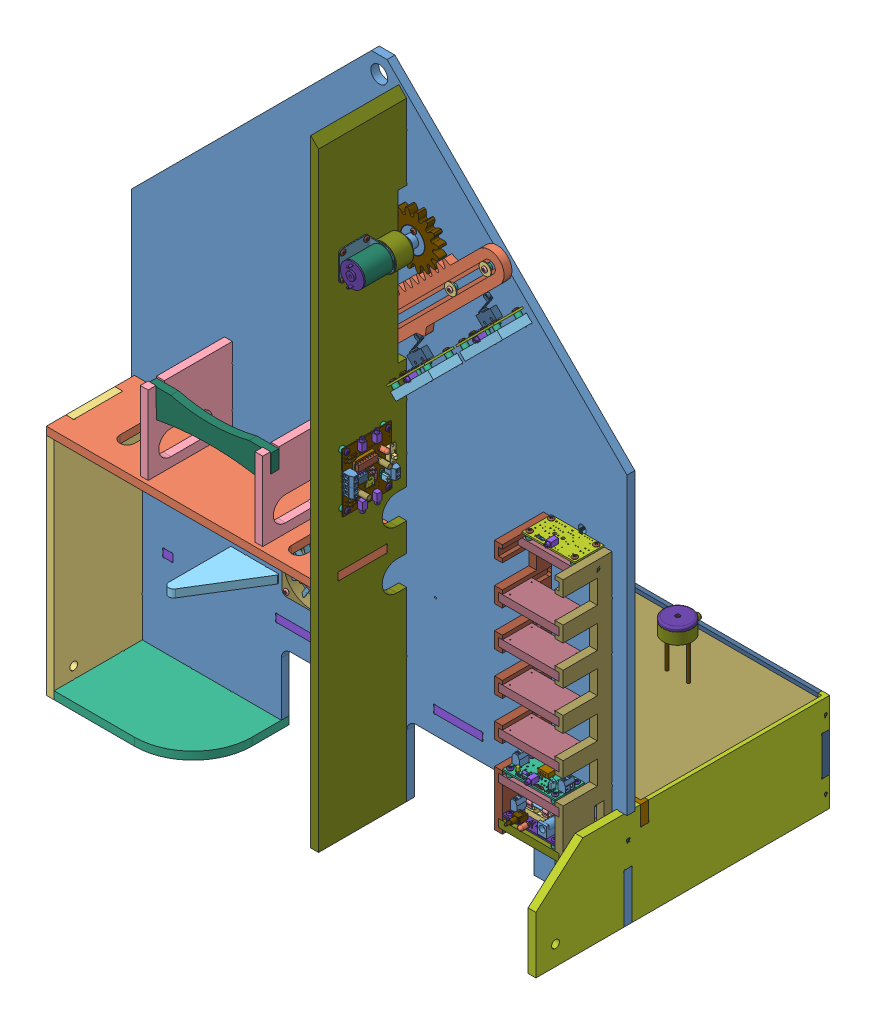
SolidWorks assembly Serre de base, configuration guillotine. Lengths in mm. (continued)
Components (placement in the parent): (continued)
- Cache Oled-2: Cache Oled [Défaut] at (-241.7989 -284.4707 -216)
- guillotine-1: guillotine [Défaut] at (-150.376 -16.7665 73.5)
- Sonde capteur humidité-1: Sonde capteur humidité [Défaut] at (349.3697 -143.9656 -111.3159) x (1 0 0) z (0 1 0) size (30.38 36.99 53.6)
  - Base capteur humidité terre-1: Base capteur humidité terre [Défaut] at (-210.4875 -4.2437 -4) size (29.6 36.6 12.37)
  - Capot capteur humidité terre-1: Capot capteur humidité terre [Défaut] at (-210.4875 -4.2437 32.3863) x (0 0 1) z (-0.999641 -0.026785 0) size (7 29.6 29.6)
  - Tige capteur humidité-1: Tige capteur humidité [Défaut] at (-221.4875 -4.2437 8) x (1 0 0) z (0 1 0) size (3 50 3)
  - Tige capteur humidité-2: Tige capteur humidité [Défaut] at (-199.4875 -4.2437 8) x (1 0 0) z (0 1 0) size (3 50 3)
  - CI capteur humidité terre-1: CI capteur humidité terre [Défaut] at (-210.4875 -4.2437 3) size (25.6 25.6 1.6)
  - Vis 2.2 x 9.5-1: Vis 2.2 x 9.5 [Défaut] at (-210.4875 -4.2437 9.6) x (0.624792 0.780791 0) z (0.780791 -0.624792 0) size (4.27 12.1 4.27)
  - Résistance 75 Kohm Pas de 10-1: Résistance 75 Kohm Pas de 10 [Défaut] at (-210.4875 -12.0088 0.7228) x (1 0 0) z (0 1 0) size (10.5 4.15 2.3)
Mates (geometry in assembly coordinates):
- Coïncidente1: coincident anti-aligned: axis of FONDINTERIEUR-1 through (57.939 191.6778 -4) axis (0 0 1); axis of Rondelle métal 3 x 12-1 through (57.939 191.6778 8.8) axis (0 0 -1)
- Coïncidente2: coincident anti-aligned: axis of Rondelle métal 3 x 12-1 through (57.939 191.6778 8.8) axis (0 0 -1); axis of VIs TC 3 x 13-1 through (57.939 191.6778 -1.7) axis (0 0 1)
- Coïncidente3: coincident anti-aligned: axis of FONDINTERIEUR-1 through (22.5836 156.3225 -4) axis (0 0 1); axis of Rondelle métal 3 x 12-2 through (22.5836 156.3225 8.8) axis (0 0 -1)
- Coïncidente4: coincident anti-aligned: axis of VIs TC 3 x 13-2 through (22.5836 156.3225 -1.7) axis (0 0 1); axis of Rondelle métal 3 x 12-2 through (22.5836 156.3225 8.8) axis (0 0 -1)
- Coïncidente5: coincident aligned: circle of VIs TC 3 x 13-2; plane of Rondelle métal 3 x 12-2 through (22.5836 156.3225 8.8) normal (0 0 1)
- Coïncidente6: coincident anti-aligned: plane of Rondelle métal 3 x 12-1 through (57.939 191.6778 8.8) normal (0 0 1); plane of VIs TC 3 x 13-1 through (57.939 191.6778 8.8) normal (0 0 -1)
- Coïncidente14: coincident anti-aligned: axis of FONDINTERIEUR-1 through (57.939 191.6778 -4) axis (0 0 1); axis of Entretoise CI-1 through (57.939 191.6778 8.1) axis (0 0 -1)
- Coïncidente15: coincident aligned: plane of FONDINTERIEUR-1 through (-297.9367 -225.0262 4) normal (0 0 1); circle of Entretoise CI-1
- Coïncidente16: coincident anti-aligned: axis of FONDINTERIEUR-1 through (22.5836 156.3225 -4) axis (0 0 1); axis of Entretoise CI-2 through (22.5836 156.3225 8.1) axis (0 0 -1)
- Coïncidente17: coincident aligned: plane of FONDINTERIEUR-1 through (-297.9367 -225.0262 4) normal (0 0 1); circle of Entretoise CI-2
- Tangent4: tangent anti-aligned: plane of Crémallière M3-3-1 through (-72.5742 65.3366 12) normal (0.707107 -0.707107 0); cylinder of Entretoise CI-2 through (22.5836 156.3225 8.1) axis (0 0 -1) radius 2.95
- Parallèle1: parallel aligned: plane of FONDINTERIEUR-1 through (-307.876 77.2771 4) normal (-0.707107 0.707107 0); plane of Crémallière M3-3-1 through (-52.7752 102.1062 12) normal (-0.707107 0.707107 0)
- Coïncidente19: coincident anti-aligned: plane of FONDINTERIEUR-1 through (-297.9367 -225.0262 4) normal (0 0 1); plane of Crémallière M3-3-1 through (65.6965 199.3646 4) normal (0 0 -1)
- Coïncidente20: coincident aligned: axis of FONDINTERIEUR-1 through (57.939 191.6778 -4) axis (0 0 1); axis of VIs TC 3 x 13-1 through (57.939 191.6778 -1.7) axis (0 0 1)
- Coïncidente21: coincident anti-aligned: plane of Crémallière M3-3-1 through (-70.4528 63.2153 8) normal (0 0 1); plane of Rondelle métal 3 x 12-1 through (57.939 191.6778 8) normal (0 0 -1)
- Coïncidente22: coincident anti-aligned: plane of Crémallière M3-3-1 through (-70.4528 63.2153 8) normal (0 0 1); plane of Rondelle métal 3 x 12-2 through (22.5836 156.3225 8) normal (0 0 -1)
- Coïncidente23: coincident anti-aligned: plane of FONDINTERIEUR-1 through (62.7794 136.4142 -4) normal (0.707107 -0.707107 0); plane of Prépa 06 module Microrupteur-1/support capteur-1 through (87.5711 161.2058 2.9393) normal (-0.707107 0.707107 0)
- Coïncidente24: coincident anti-aligned: plane of FONDINTERIEUR-1 through (96.8921 167.5269 -4) normal (-0.707107 -0.707107 0); plane of Prépa 06 module Microrupteur-1/support capteur-1 through (95.3921 169.0269 -4) normal (0.707107 0.707107 0)
- Coïncidente25: coincident aligned: plane of FONDINTERIEUR-1 through (-297.9367 -225.0262 -4) normal (0 0 -1); plane of Prépa 06 module Microrupteur-1/support capteur-1 through (95.3921 169.0269 -4) normal (0 0 -1)
- Coïncidente26: coincident anti-aligned: plane of FONDINTERIEUR-1 through (-7.9312 65.7035 -4) normal (0.707107 -0.707107 0); plane of Prépa 06 module Microrupteur-2/support capteur-1 through (16.8604 90.4952 2.9393) normal (-0.707107 0.707107 0)
- Coïncidente27: coincident anti-aligned: plane of FONDINTERIEUR-1 through (26.1815 96.8162 -4) normal (-0.707107 -0.707107 0); plane of Prépa 06 module Microrupteur-2/support capteur-1 through (24.6815 98.3162 -4) normal (0.707107 0.707107 0)
- Coïncidente28: coincident aligned: plane of FONDINTERIEUR-1 through (-297.9367 -225.0262 -4) normal (0 0 -1); plane of Prépa 06 module Microrupteur-2/support capteur-1 through (24.6815 98.3162 -4) normal (0 0 -1)
- Coïncidente29: coincident anti-aligned: axis of FONDINTERIEUR-1 through (-138.876 -138.9656 -4) axis (0 0 1); axis of Ventilateur-1/Cage ventilateur-1 through (-138.876 -138.9656 14.4) axis (0 0 -1)
- Coïncidente30: coincident anti-aligned: axis of FONDINTERIEUR-1 through (-88.876 -138.9656 -4) axis (0 0 1); axis of Ventilateur-1/Cage ventilateur-1 through (-88.876 -138.9656 14.4) axis (0 0 -1)
- Coïncidente31: coincident: plane of FONDINTERIEUR-1 through (-297.9367 -225.0262 4) normal (0 0 1); line of Ventilateur-1/Cage ventilateur-1 through (-143.876 -138.9656 4) axis (0 -1 0)
- Coïncidente32: coincident anti-aligned: axis of Ventilateur-1/Cage ventilateur-1 through (-138.876 -138.9656 14.4) axis (0 0 -1); axis of VIs TC 3 x 13-4 through (-138.876 -138.9656 3.9) axis (0 0 1)
- Coïncidente33: coincident anti-aligned: axis of Ventilateur-1/Cage ventilateur-1 through (-88.876 -138.9656 14.4) axis (0 0 -1); axis of VIs TC 3 x 13-6 through (-88.876 -138.9656 3.9) axis (0 0 1)
- Coïncidente34: coincident anti-aligned: axis of Ventilateur-1/Cage ventilateur-1 through (-88.876 -188.9656 14.4) axis (0 0 -1); axis of VIs TC 3 x 13-7 through (-88.876 -188.9656 3.9) axis (0 0 1)
- Coïncidente35: coincident anti-aligned: axis of Ventilateur-1/Cage ventilateur-1 through (-138.876 -188.9656 14.4) axis (0 0 -1); axis of VIs TC 3 x 13-8 through (-138.876 -188.9656 3.9) axis (0 0 1)
- Coïncidente36: coincident aligned: plane of Ventilateur-1/Cage ventilateur-1 through (-88.876 -138.9656 14.4) normal (0 0 1); circle of VIs TC 3 x 13-8
- Coïncidente37: coincident aligned: plane of Ventilateur-1/Cage ventilateur-1 through (-88.876 -138.9656 14.4) normal (0 0 1); circle of VIs TC 3 x 13-4
- Coïncidente38: coincident aligned: plane of Ventilateur-1/Cage ventilateur-1 through (-88.876 -138.9656 14.4) normal (0 0 1); circle of VIs TC 3 x 13-6
- Coïncidente39: coincident aligned: plane of Ventilateur-1/Cage ventilateur-1 through (-88.876 -138.9656 14.4) normal (0 0 1); circle of VIs TC 3 x 13-7
- Coïncidente40: coincident aligned: axis of FONDINTERIEUR-1 through (8.418 76.3959 4) axis (0 0 -1); axis of VIS TORCX TF 3 X 19-2 through (8.418 76.3959 12.4885) axis (0 0 -1)
- Coïncidente41: coincident aligned: plane of FONDINTERIEUR-1 through (-297.9367 -225.0262 -4) normal (0 0 -1); plane of VIS TORCX TF 3 X 19-2 through (7.3455 78.9824 -4) normal (0 0 -1)
- Coïncidente42: coincident aligned: axis of FONDINTERIEUR-1 through (79.1287 147.1066 4) axis (0 0 -1); axis of VIS TORCX TF 3 X 19-1 through (79.1287 147.1066 12.4885) axis (0 0 -1)
- Coïncidente43: coincident aligned: plane of FONDINTERIEUR-1 through (-297.9367 -225.0262 -4) normal (0 0 -1); plane of VIS TORCX TF 3 X 19-1 through (78.0561 149.693 -4) normal (0 0 -1)
- Coïncidente44: coincident anti-aligned: plane of FONDINTERIEUR-1 through (-26.876 223.1558 -4) normal (-1 0 0); plane of Prépa 02 renfort arrière-1/renfortarriere-1 through (-26.876 272.0951 2.9393) normal (1 0 0)
- Coïncidente45: coincident anti-aligned: plane of FONDINTERIEUR-1 through (-28.9973 271.0344 -4) normal (0 -1 0); plane of Prépa 02 renfort arrière-1/renfortarriere-1 through (-26.876 271.0344 -4) normal (0 1 0)
- Coïncidente46: coincident aligned: plane of FONDINTERIEUR-1 through (-297.9367 -225.0262 -4) normal (0 0 -1); plane of Prépa 02 renfort arrière-1/renfortarriere-1 through (-26.876 221.1086 -4) normal (0 0 -1)
- Coïncidente47: coincident anti-aligned: plane of FONDINTERIEUR-1 through (-56.9973 -85.9656 -4) normal (0 -1 0); plane of étagèrebrumi-1 through (-297.9367 -85.9656 72.872) normal (0 1 0)
- Coïncidente48: coincident anti-aligned: plane of FONDINTERIEUR-1 through (-54.876 -88.0869 -4) normal (-1 0 0); plane of étagèrebrumi-1 through (-54.876 -85.9656 1.8787) normal (1 0 0)
- Coïncidente49: coincident aligned: plane of FONDINTERIEUR-1 through (-297.9367 -225.0262 -4) normal (0 0 -1); plane of étagèrebrumi-1 through (-54.876 -85.9656 -4) normal (0 0 -1)
- Coïncidente50: coincident anti-aligned: axis of FONDINTERIEUR-1 through (-30.876 -315.9656 -4) axis (0 0 1); axis of VIS TORCX TF 3 X 19-3 through (-30.876 -315.9656 12.4885) axis (0 0 -1)
- Coïncidente51: coincident aligned: plane of FONDINTERIEUR-1 through (-297.9367 -225.0262 -4) normal (0 0 -1); plane of VIS TORCX TF 3 X 19-3 through (-31.2492 -313.1905 -4) normal (0 0 -1)
- Coïncidente52: coincident anti-aligned: axis of FONDINTERIEUR-1 through (-30.876 -274.5499 -4) axis (0 0 1); axis of VIS TORCX TF 3 X 19-4 through (-30.876 -274.5499 12.4885) axis (0 0 -1)
- Coïncidente53: coincident aligned: plane of FONDINTERIEUR-1 through (-297.9367 -225.0262 -4) normal (0 0 -1); plane of VIS TORCX TF 3 X 19-4 through (-31.2492 -271.7749 -4) normal (0 0 -1)
- Coïncidente54: coincident anti-aligned: axis of FONDINTERIEUR-1 through (-169.876 -89.9656 -4) axis (0 0 1); axis of VIS TORCX TF 3 X 19-5 through (-169.876 -89.9656 12.4885) axis (0 0 -1)
- Coïncidente55: coincident aligned: plane of FONDINTERIEUR-1 through (-297.9367 -225.0262 -4) normal (0 0 -1); plane of VIS TORCX TF 3 X 19-5 through (-170.2492 -87.1905 -4) normal (0 0 -1)
- Coïncidente56: coincident anti-aligned: axis of FONDINTERIEUR-1 through (-30.876 -27.0369 -4) axis (0 0 1); axis of VIS TORCX TF 3 X 19-6 through (-30.876 -27.0369 12.4885) axis (0 0 -1)
- Coïncidente57: coincident aligned: plane of FONDINTERIEUR-1 through (-297.9367 -225.0262 -4) normal (0 0 -1); plane of VIS TORCX TF 3 X 19-6 through (-31.2492 -24.2619 -4) normal (0 0 -1)
- Coïncidente58: coincident anti-aligned: axis of FONDINTERIEUR-1 through (-30.876 278.5344 -4) axis (0 0 1); axis of VIS TORCX TF 3 X 19-7 through (-30.876 278.5344 12.4885) axis (0 0 -1)
- Coïncidente59: coincident aligned: plane of FONDINTERIEUR-1 through (-297.9367 -225.0262 -4) normal (0 0 -1); plane of VIS TORCX TF 3 X 19-7 through (-31.2492 281.3095 -4) normal (0 0 -1)
- Coïncidente60: coincident anti-aligned: plane of FONDINTERIEUR-1 through (-296.876 -226.0869 4) normal (-1 0 0); plane of Coté gauche serre-1 through (-296.876 -275.0426 -2.9402) normal (1 0 0)
- Coïncidente61: coincident anti-aligned: plane of FONDINTERIEUR-1 through (-298.9973 -273.9656 4) normal (0 1 0); plane of Coté gauche serre-1 through (-296.876 -273.9656 1.8944) normal (0 -1 0)
- Coïncidente62: coincident anti-aligned: plane of FONDINTERIEUR-1 through (-297.9367 -225.0262 -4) normal (0 0 -1); plane of Coté gauche serre-1 through (-296.876 -323.9656 -4) normal (0 0 1)
- Coïncidente63: coincident anti-aligned: plane of FONDINTERIEUR-1 through (-154.876 -315.9656 -4) normal (0 -1 0); plane of suportbloceau-1 through (-297.9367 -315.9656 75.0607) normal (0 1 0)
- Coïncidente64: coincident anti-aligned: plane of FONDINTERIEUR-1 through (-204.876 -318.0869 -4) normal (1 0 0); plane of suportbloceau-1 through (-204.876 -315.9656 -4) normal (-1 0 0)
- Coïncidente65: coincident aligned: plane of FONDINTERIEUR-1 through (-297.9367 -225.0262 -4) normal (0 0 -1); plane of suportbloceau-1 through (-154.876 -315.9656 -4) normal (0 0 -1)
- Coïncidente66: coincident anti-aligned: plane of FONDINTERIEUR-1 through (-95.876 -28.0869 4) normal (1 0 0); plane of Coté support brumisateur-1 through (-95.876 -24.9049 2.9393) normal (-1 0 0)
- Coïncidente67: coincident anti-aligned: plane of FONDINTERIEUR-1 through (-89.9973 -65.9656 4) normal (0 1 0); plane of Coté support brumisateur-1 through (-95.876 -65.9656 -4) normal (0 -1 0)
- Coïncidente68: coincident aligned: plane of FONDINTERIEUR-1 through (-297.9367 -225.0262 -4) normal (0 0 -1); plane of Coté support brumisateur-1 through (-95.876 -25.9656 -4) normal (0 0 -1)
- Coïncidente69: coincident anti-aligned: plane of FONDINTERIEUR-1 through (-212.876 -28.0869 4) normal (1 0 0); plane of Coté support brumisateur-2 through (-212.876 -24.9049 2.9393) normal (-1 0 0)
- Coïncidente70: coincident anti-aligned: plane of FONDINTERIEUR-1 through (-210.7547 -65.9656 4) normal (0 1 0); plane of Coté support brumisateur-2 through (-212.876 -65.9656 -4) normal (0 -1 0)
- Coïncidente71: coincident aligned: plane of FONDINTERIEUR-1 through (-297.9367 -225.0262 -4) normal (0 0 -1); plane of Coté support brumisateur-2 through (-212.876 -25.9656 -4) normal (0 0 -1)
- Coïncidente72: coincident anti-aligned: plane of FONDINTERIEUR-1 through (-189.2547 -195.9656 -4) normal (0 1 0); plane of Renfort bidon-1 through (-192.4367 -195.9656 2.9393) normal (0 -1 0)
- Coïncidente73: coincident anti-aligned: plane of FONDINTERIEUR-1 through (-191.376 -190.0869 -4) normal (1 0 0); plane of Renfort bidon-1 through (-191.376 -187.9656 1.8787) normal (-1 0 0)
- Coïncidente74: coincident aligned: plane of FONDINTERIEUR-1 through (-297.9367 -225.0262 -4) normal (0 0 -1); plane of Renfort bidon-1 through (-191.376 -187.9656 -4) normal (0 0 -1)
- Coïncidente75: coincident aligned: axis of FONDINTERIEUR-1 through (-198.876 -191.9656 4) axis (0 0 -1); axis of VIS TORCX TF 3 X 19-12 through (-198.876 -191.9656 12.4885) axis (0 0 -1)
- Coïncidente76: coincident aligned: plane of FONDINTERIEUR-1 through (-297.9367 -225.0262 -4) normal (0 0 -1); plane of VIS TORCX TF 3 X 19-12 through (-199.9485 -189.3791 -4) normal (0 0 -1)
- Coïncidente77: coincident aligned: axis of FONDINTERIEUR-1 through (-164.4919 -191.9656 4) axis (0 0 -1); axis of VIS TORCX TF 3 X 19-13 through (-164.4919 -191.9656 12.4885) axis (0 0 -1)
- Coïncidente78: coincident aligned: plane of FONDINTERIEUR-1 through (-297.9367 -225.0262 -4) normal (0 0 -1); plane of VIS TORCX TF 3 X 19-13 through (-165.5644 -189.3791 -4) normal (0 0 -1)
- Coïncidente79: coincident aligned: axis of FONDINTERIEUR-1 through (-208.876 -75.9656 4) axis (0 0 -1); axis of VIS TORCX TF 3 X 19-14 through (-208.876 -75.9656 12.4885) axis (0 0 -1)
- Coïncidente80: coincident aligned: plane of FONDINTERIEUR-1 through (-297.9367 -225.0262 -4) normal (0 0 -1); plane of VIS TORCX TF 3 X 19-14 through (-209.9485 -73.3791 -4) normal (0 0 -1)
- Coïncidente81: coincident aligned: axis of FONDINTERIEUR-1 through (-208.876 -16.4656 4) axis (0 0 -1); axis of VIS TORCX TF 3 X 19-15 through (-208.876 -16.4656 12.4885) axis (0 0 -1)
- Coïncidente82: coincident aligned: plane of FONDINTERIEUR-1 through (-297.9367 -225.0262 -4) normal (0 0 -1); plane of VIS TORCX TF 3 X 19-15 through (-209.9485 -13.8791 -4) normal (0 0 -1)
- Coïncidente83: coincident aligned: axis of FONDINTERIEUR-1 through (-91.876 -75.9656 4) axis (0 0 -1); axis of VIS TORCX TF 3 X 19-16 through (-91.876 -75.9656 12.4885) axis (0 0 -1)
- Coïncidente84: coincident aligned: plane of FONDINTERIEUR-1 through (-297.9367 -225.0262 -4) normal (0 0 -1); plane of VIS TORCX TF 3 X 19-16 through (-92.9485 -73.3791 -4) normal (0 0 -1)
- Coïncidente85: coincident aligned: axis of FONDINTERIEUR-1 through (-91.876 -15.9656 4) axis (0 0 -1); axis of VIS TORCX TF 3 X 19-17 through (-91.876 -15.9656 12.4885) axis (0 0 -1)
- Coïncidente86: coincident aligned: plane of FONDINTERIEUR-1 through (-297.9367 -225.0262 -4) normal (0 0 -1); plane of VIS TORCX TF 3 X 19-17 through (-92.9485 -13.3791 -4) normal (0 0 -1)
- Coïncidente87: coincident aligned: axis of Coté gauche serre-1 through (-296.876 -89.9656 48.9996) axis (-1 0 0); axis of VIS TORCX TF 3 X 19-18 through (-288.3875 -89.9656 48.9996) axis (-1 0 0)
- Coïncidente88: coincident aligned: plane of Coté gauche serre-1 through (-304.876 -275.0426 -2.9402) normal (-1 0 0); plane of VIS TORCX TF 3 X 19-18 through (-304.876 -87.1656 48.9996) normal (-1 0 0)
- Coïncidente89: coincident aligned: axis of Coté gauche serre-1 through (-296.876 -248.9656 -0.0009) axis (-1 0 0); axis of VIS TORCX TF 3 X 19-25 through (-288.3875 -248.9656 -0.0009) axis (-1 0 0)
- Coïncidente90: coincident aligned: plane of Coté gauche serre-1 through (-304.876 -275.0426 -2.9402) normal (-1 0 0); plane of VIS TORCX TF 3 X 19-25 through (-304.876 -246.1656 -0.0009) normal (-1 0 0)
- Coïncidente91: coincident aligned: axis of suportbloceau-1 through (-300.876 -315.9656 49) axis (0 -1 0); axis of VIS TORCX TF 3 X 19-26 through (-300.876 -307.477 49) axis (0 -1 0)
- Coïncidente92: coincident aligned: plane of suportbloceau-1 through (-297.9367 -323.9656 75.0607) normal (0 -1 0); plane of VIS TORCX TF 3 X 19-26 through (-299.1327 -323.9656 51.1911) normal (0 -1 0)
- Coïncidente93: coincident aligned: axis of suportbloceau-1 through (-271.876 -315.9656 0) axis (0 -1 0); axis of VIS TORCX TF 3 X 19-29 through (-271.876 -307.477 0) axis (0 -1 0)
- Coïncidente94: coincident aligned: plane of suportbloceau-1 through (-297.9367 -323.9656 75.0607) normal (0 -1 0); plane of VIS TORCX TF 3 X 19-29 through (-270.1327 -323.9656 2.1911) normal (0 -1 0)
- Coïncidente95: coincident aligned: axis of suportbloceau-1 through (-179.876 -315.9656 0) axis (0 -1 0); axis of VIS TORCX TF 3 X 19-30 through (-179.876 -307.477 0) axis (0 -1 0)
- Coïncidente96: coincident aligned: plane of suportbloceau-1 through (-297.9367 -323.9656 75.0607) normal (0 -1 0); plane of VIS TORCX TF 3 X 19-30 through (-178.1327 -323.9656 2.1911) normal (0 -1 0)
- Coïncidente103: coincident anti-aligned: plane of FONDINTERIEUR-1 through (187.124 -226.0869 4) normal (1 0 0); plane of Coté droit serre-1 through (187.124 -275.0262 -2.9393) normal (-1 0 0)
- Coïncidente104: coincident anti-aligned: plane of FONDINTERIEUR-1 through (195.124 -223.9656 4) normal (0 -1 0); plane of Coté droit serre-1 through (195.124 -223.9656 46) normal (0 1 0)
- Coïncidente105: coincident anti-aligned: plane of FONDINTERIEUR-1 through (-297.9367 -225.0262 -4) normal (0 0 -1); plane of Coté droit serre-1 through (195.124 -323.9656 -4) normal (0 0 1)
- Coïncidente114: coincident anti-aligned: axis of Coté droit serre-1 through (195.124 -248.9656 0) axis (-1 0 0); axis of VIS TORCX TF 3 X 19-35 through (178.6355 -248.9656 0) axis (1 0 0)
- Coïncidente115: coincident aligned: plane of Coté droit serre-1 through (195.124 -275.0262 -2.9393) normal (1 0 0); plane of VIS TORCX TF 3 X 19-35 through (195.124 -246.2177 -0.5377) normal (1 0 0)
- Coïncidente116: coincident anti-aligned: plane of FONDINTERIEUR-1 through (48.6689 -231.9656 -4) normal (0 1 0); plane of Poutre fond-1 through (-276.7874 -231.9656 -2.9393) normal (0 -1 0)
- Coïncidente117: coincident anti-aligned: plane of FONDINTERIEUR-1 through (0.7902 -229.8442 -4) normal (1 0 0); plane of Poutre fond-1 through (0.7902 -223.9656 4) normal (-1 0 0)
- Coïncidente118: coincident anti-aligned: plane of FONDINTERIEUR-1 through (-297.9367 -225.0262 -4) normal (0 0 -1); plane of Poutre fond-1 through (-108.4209 -223.9656 -4) normal (0 0 1)
- Coïncidente119: coincident aligned: axis of FONDINTERIEUR-1 through (103.3825 -227.9656 -4) axis (0 0 1); axis of VIS TORCX TF 3 X 19-49 through (103.3825 -227.9656 -12.4885) axis (0 0 1)
- Coïncidente120: coincident aligned: plane of FONDINTERIEUR-1 through (-297.9367 -225.0262 4) normal (0 0 1); plane of VIS TORCX TF 3 X 19-49 through (103.3825 -225.1656 4) normal (0 0 1)
- Coïncidente121: coincident aligned: axis of FONDINTERIEUR-1 through (-54.876 -227.9656 -4) axis (0 0 1); axis of VIS TORCX TF 3 X 19-37 through (-54.876 -227.9656 -12.4885) axis (0 0 1)
- Coïncidente122: coincident aligned: plane of FONDINTERIEUR-1 through (-297.9367 -225.0262 4) normal (0 0 1); plane of VIS TORCX TF 3 X 19-37 through (-54.876 -225.1656 4) normal (0 0 1)
- Coïncidente124: coincident aligned: axis of FONDINTERIEUR-1 through (-213.1345 -227.9656 -4) axis (0 0 1); axis of VIS TORCX TF 3 X 19-36 through (-213.1345 -227.9656 -12.4885) axis (0 0 1)
- Coïncidente125: coincident aligned: plane of FONDINTERIEUR-1 through (-297.9367 -225.0262 4) normal (0 0 1); plane of VIS TORCX TF 3 X 19-36 through (-213.1345 -225.1656 4) normal (0 0 1)
- Coïncidente126: coincident anti-aligned: plane of Poutre fond-1 through (-296.876 -223.9656 -13) normal (0 0 -1); plane of Poutre plateau-1 through (79.7388 -229.6404 -13) normal (0 0 1)
- Coïncidente127: coincident aligned: plane of Coté droit serre-1 through (195.124 -275.0262 -2.9393) normal (1 0 0); plane of Poutre plateau-1 through (195.124 -223.9656 -21) normal (1 0 0)
- Coïncidente128: coincident anti-aligned: plane of Coté droit serre-1 through (195.124 -243.9656 -18.9697) normal (0 1 0); plane of Poutre plateau-1 through (195.124 -243.9656 -21) normal (0 -1 0)
- Coïncidente129: coincident anti-aligned: plane of Coté droit serre-1 through (195.124 -291.8442 -198) normal (0 0 -1); plane of façadeporteplateau-1 through (188.1847 -295.0262 -198) normal (0 0 1)
- Coïncidente130: coincident aligned: plane of Coté droit serre-1 through (195.124 -275.0262 -2.9393) normal (1 0 0); plane of façadeporteplateau-1 through (195.124 -253.9656 -198) normal (1 0 0)
- Coïncidente131: coincident aligned: plane of Coté droit serre-1 through (195.124 -223.9656 -21.091) normal (0 1 0); plane of façadeporteplateau-1 through (-296.876 -223.9656 -198) normal (0 1 0)
- Coïncidente132: coincident anti-aligned: axis of Coté droit serre-1 through (195.124 -238.9656 -202) axis (-1 0 0); axis of VIS TORCX TF 3 X 19-40 through (178.6355 -238.9656 -202) axis (1 0 0)
- Coïncidente133: coincident aligned: plane of Coté droit serre-1 through (195.124 -275.0262 -2.9393) normal (1 0 0); plane of VIS TORCX TF 3 X 19-40 through (195.124 -236.1656 -202) normal (1 0 0)
- Coïncidente134: coincident anti-aligned: axis of Coté droit serre-1 through (195.124 -308.9656 -202) axis (-1 0 0); axis of VIS TORCX TF 3 X 19-39 through (178.6355 -308.9656 -202) axis (1 0 0)
- Coïncidente135: coincident aligned: plane of Coté droit serre-1 through (195.124 -275.0262 -2.9393) normal (1 0 0); plane of VIS TORCX TF 3 X 19-39 through (195.124 -306.1656 -202) normal (1 0 0)
- Coïncidente136: coincident aligned: axis of façadeporteplateau-1 through (191.124 -273.9656 -198) axis (0 0 -1); axis of VIS TORCX TF 3 X 19-38 through (191.124 -273.9656 -189.5115) axis (0 0 -1)
- Coïncidente137: coincident aligned: plane of façadeporteplateau-1 through (188.1847 -295.0262 -206) normal (0 0 -1); plane of VIS TORCX TF 3 X 19-38 through (190.0515 -271.3791 -206) normal (0 0 -1)
- Coïncidente138: coincident aligned: axis of façadeporteplateau-1 through (-300.876 -273.9656 -198) axis (0 0 -1); axis of VIS TORCX TF 3 X 19-43 through (-300.876 -273.9656 -189.5115) axis (0 0 -1)
- Coïncidente139: coincident aligned: plane of façadeporteplateau-1 through (188.1847 -295.0262 -206) normal (0 0 -1); plane of VIS TORCX TF 3 X 19-43 through (-301.9485 -271.3791 -206) normal (0 0 -1)
- Coïncidente140: coincident aligned: axis of Coté gauche serre-1 through (-296.876 -238.9737 -202) axis (-1 0 0); axis of VIS TORCX TF 3 X 19-44 through (-288.3875 -238.9737 -202) axis (-1 0 0)
- Coïncidente141: coincident aligned: plane of Coté gauche serre-1 through (-304.876 -275.0426 -2.9402) normal (-1 0 0); plane of VIS TORCX TF 3 X 19-44 through (-304.876 -236.1737 -202) normal (-1 0 0)
- Coïncidente142: coincident aligned: axis of Coté gauche serre-1 through (-296.876 -308.9656 -202) axis (-1 0 0); axis of VIS TORCX TF 3 X 19-45 through (-288.3875 -308.9656 -202) axis (-1 0 0)
- Coïncidente143: coincident aligned: plane of Coté gauche serre-1 through (-304.876 -275.0426 -2.9402) normal (-1 0 0); plane of VIS TORCX TF 3 X 19-45 through (-304.876 -306.1656 -202) normal (-1 0 0)
- Coïncidente144: coincident anti-aligned: plane of FONDINTERIEUR-1 through (112.8547 -40.3939 -4) normal (1 0 0); plane of Sous ensemble Rack module-1/rack coté gauche-1 through (112.8547 -36.9223 2.9393) normal (-1 0 0)
- Coïncidente145: coincident anti-aligned: plane of FONDINTERIEUR-1 through (176.9761 -37.9656 -4) normal (0 -1 0); plane of Sous ensemble Rack module-1/rack coté droit-1 through (182.8547 -37.9656 1.8787) normal (0 1 0)
- Coïncidente146: coincident aligned: plane of FONDINTERIEUR-1 through (-297.9367 -225.0262 -4) normal (0 0 -1); plane of Sous ensemble Rack module-1/rack coté droit-1 through (182.8547 -37.9656 -4) normal (0 0 -1)
- Coïncidente147: coincident aligned: axis of FONDINTERIEUR-1 through (178.8547 -145.9656 4) axis (0 0 -1); axis of VIS TORCX TF 3 X 19-50 through (178.8547 -145.9656 12.4885) axis (0 0 -1)
- Coïncidente148: coincident aligned: plane of FONDINTERIEUR-1 through (-297.9367 -225.0262 -4) normal (0 0 -1); plane of VIS TORCX TF 3 X 19-50 through (177.7822 -143.3791 -4) normal (0 0 -1)
- Coïncidente149: coincident aligned: axis of FONDINTERIEUR-1 through (116.8547 -145.9656 4) axis (0 0 -1); axis of VIS TORCX TF 3 X 19-51 through (116.8547 -145.9656 12.4885) axis (0 0 -1)
- Coïncidente150: coincident aligned: plane of FONDINTERIEUR-1 through (-297.9367 -225.0262 -4) normal (0 0 -1); plane of VIS TORCX TF 3 X 19-51 through (115.7822 -143.3791 -4) normal (0 0 -1)
- Coïncidente151: coincident anti-aligned: axis of FONDINTERIEUR-1 through (178.8547 -7.9656 -4) axis (0 0 1); axis of VIS TORCX TF 3 X 19-52 through (178.8547 -7.9656 12.4885) axis (0 0 -1)
- Coïncidente152: coincident aligned: plane of FONDINTERIEUR-1 through (-297.9367 -225.0262 -4) normal (0 0 -1); plane of VIS TORCX TF 3 X 19-52 through (177.7822 -5.3791 -4) normal (0 0 -1)
- Coïncidente153: coincident anti-aligned: axis of FONDINTERIEUR-1 through (116.8547 -7.9656 -4) axis (0 0 1); axis of VIS TORCX TF 3 X 19-53 through (116.8547 -7.9656 12.4885) axis (0 0 -1)
- Coïncidente154: coincident aligned: plane of FONDINTERIEUR-1 through (-297.9367 -225.0262 -4) normal (0 0 -1); plane of VIS TORCX TF 3 X 19-53 through (115.7822 -5.3791 -4) normal (0 0 -1)
- Coïncidente163: coincident aligned: axis of FONDINTERIEUR-1 through (-255.126 -66.1655 -4) axis (0 0 1); axis of Sous ensemble Arrosage-1/Tuyau gouteur-1 through (-255.126 -66.1655 -11.25) axis (0 0 1)
- Coïncidente164: coincident anti-aligned: plane of suportbloceau-1 through (-297.9367 -315.9656 75.0607) normal (0 1 0); plane of Sous ensemble Arrosage-1/Reservoir 1,25L-1 through (-272.5 -315.9655 45.1435) normal (0 -1 0)
- Coïncidente168: coincident anti-aligned: plane of FONDINTERIEUR-1 through (-297.9367 -225.0262 4) normal (0 0 1); plane of Sous ensemble Arrosage-1/Reservoir 1,25L-1 through (-299.876 -315.9655 4) normal (0 0 -1)
- Coïncidente169: coincident anti-aligned: plane of Coté droit serre-1 through (191.124 -234.9049 -200.9393) normal (-1 0 0); plane of plateau base-1 through (191.124 -227.9656 -202) normal (1 0 0)
- Coïncidente170: coincident anti-aligned: plane of Coté droit serre-1 through (191.124 -235.9656 -199.8787) normal (0 1 0); plane of plateau base-1 through (-230.7684 -235.9656 -41.3241) normal (0 -1 0)
- Coïncidente173: coincident anti-aligned: plane of Poutre plateau-1 through (79.7388 -229.6404 -17) normal (0 0 -1); plane of plateau base-1 through (-300.876 -227.9656 -17) normal (0 0 1)
- Coïncidente178: coincident anti-aligned: axis of FONDINTERIEUR-1 through (152.3558 6.7126 -4) axis (0 0 1); axis of fondcuivré-1 through (152.3558 6.7126 -4) axis (0 0 -1)
- Coïncidente179: coincident anti-aligned: plane of FONDINTERIEUR-1 through (-297.9367 -225.0262 -4) normal (0 0 -1); plane of fondcuivré-1 through (-208.3657 -251.1382 -4) normal (0 0 1)
- Parallèle5: parallel anti-aligned: line of FONDINTERIEUR-1 through (-62.876 322.2771 -4) axis (1 0 0); line of fondcuivré-1 through (-29.876 291.0344 -5) axis (-1 0 0)
- Coïncidente180: coincident anti-aligned: plane of façadeporteplateau-1 through (188.1847 -295.0262 -206) normal (0 0 -1); plane of Capot complet-1/Capotfaçade-1 through (-305.9367 -222.9049 -206) normal (0 0 1)
- Coïncidente181: coincident aligned: plane of façadeporteplateau-1 through (-296.876 -323.9656 -198) normal (0 -1 0); plane of Capot complet-1/Capotfaçade-1 through (-312.876 -323.9656 -206) normal (0 -1 0)
- Coïncidente182: coincident anti-aligned: line of Coté droit serre-1 through (195.124 -323.9656 -4) axis (0 0 -1); line of Capot complet-1/Capot coté droit-1 through (195.124 -323.9656 -206) axis (0 0 1)
- Coïncidente185: coincident anti-aligned: plane of Capot complet-1/Capotfaçade-1 through (-305.9367 -222.9049 -214) normal (0 0 -1); plane of Cache Oled-2 through (-241.7989 -284.4707 -214) normal (0 0 1)
- Coïncidente186: coincident aligned: line of guillotine-1 through (-87.876 -25.9656 81.5) axis (0 0 -1); line of Coté support brumisateur-1 through (-87.876 -25.9656 82) axis (0 0 -1)
- Coïncidente187: coincident aligned: plane of Coté support brumisateur-1 through (-87.876 -24.9049 2.9393) normal (1 0 0); plane of guillotine-1 through (-87.876 -7.5675 81.5) normal (1 0 0)
- Coïncidente189: coincident anti-aligned: plane of Coté support brumisateur-1 through (-95.876 -25.9656 73.5) normal (0 0 1); plane of guillotine-1 through (-150.376 149.9325 73.5) normal (0 0 -1)
- Distance1: distance = 80 mm anti-aligned: plane of Sonde capteur humidité-1/Base capteur humidité terre-1 through (138.8822 -147.9656 -107.0722) normal (0 -1 0); plane of plateau base-1 through (-230.7684 -227.9656 -41.3241) normal (0 1 0)
